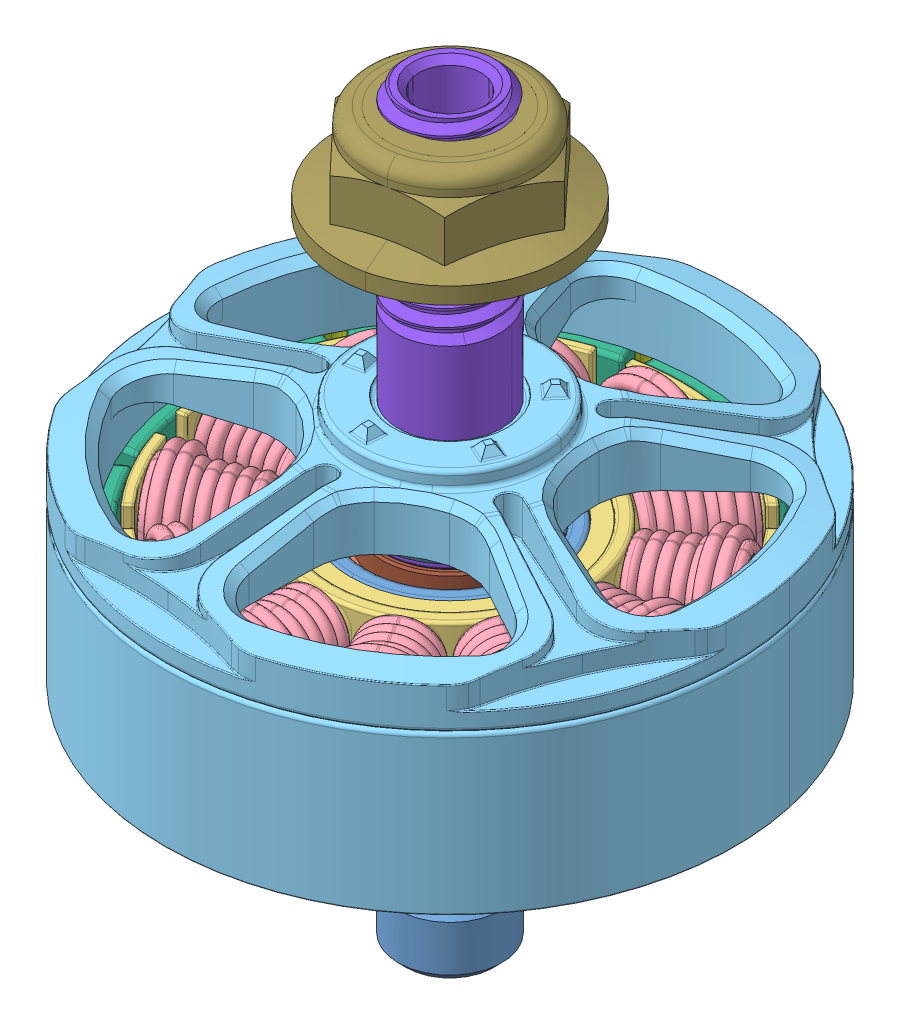
SolidWorks assembly EMAX RSII-2206 2300kv, configuration Default. Lengths in mm.
Overall size (32.76 30.2 32.81).
28 component instances, 13 part files, 0 mates.
Components (placement in the parent):
- EMAX RSII-2206 2300kv.STEP-1: EMAX RSII-2206 2300kv.STEP [Default] at origin size (61.91 30.2 32.81)
  - STATOR RSII-2206.STEP-1: STATOR RSII-2206.STEP [Default] at origin size (22.5 13.11 22.5)
    - STATOR BASE RSII-2206.STEP-1: STATOR BASE RSII-2206.STEP [Default] at origin size (16.31 12 16.31)
    - 3x8x4mm BEARING.STEP-1: 3x8x4mm BEARING.STEP [Default] at (0 5.3 0) x (1 0 0) z (0 0 -1) size (8 3 8)
    - 3x8x4mm BEARING.STEP-2: 3x8x4mm BEARING.STEP [Default] at (0 11 0) x (-0.982082 0 -0.188455) z (-0.188455 0 0.982082) size (8 3 8)
    - STATOR SLEEVE RSII-2206.STEP-1: STATOR SLEEVE RSII-2206.STEP [Default] at (0 5.5 0) size (22.5 6.65 22.5)
    - WINDING RSII-2206.STEP-1: WINDING RSII-2206.STEP [Default] at (8.5609 8.825 0) size (4.26 8.58 4.68)
    - WINDING RSII-2206.STEP-2: WINDING RSII-2206.STEP [Default] at (7.414 8.825 4.2805) x (0.866025 0 0.5) z (-0.5 0 0.866025) size (4.26 8.58 4.68)
    - WINDING RSII-2206.STEP-3: WINDING RSII-2206.STEP [Default] at (4.2805 8.825 7.414) x (0.5 0 0.866025) z (-0.866025 0 0.5) size (4.26 8.58 4.68)
    - WINDING RSII-2206.STEP-4: WINDING RSII-2206.STEP [Default] at (0 8.825 8.5609) x (0 0 1) z (-1 0 0) size (4.26 8.58 4.68)
    - WINDING RSII-2206.STEP-5: WINDING RSII-2206.STEP [Default] at (-4.2805 8.825 7.414) x (-0.5 0 0.866025) z (-0.866025 0 -0.5) size (4.26 8.58 4.68)
    - WINDING RSII-2206.STEP-6: WINDING RSII-2206.STEP [Default] at (-7.414 8.825 4.2805) x (-0.866025 0 0.5) z (-0.5 0 -0.866025) size (4.26 8.58 4.68)
    - WINDING RSII-2206.STEP-7: WINDING RSII-2206.STEP [Default] at (-8.5609 8.825 0) x (-1 0 0) z (0 0 -1) size (4.26 8.58 4.68)
    - WINDING RSII-2206.STEP-8: WINDING RSII-2206.STEP [Default] at (-7.414 8.825 -4.2805) x (-0.866025 0 -0.5) z (0.5 0 -0.866025) size (4.26 8.58 4.68)
    - WINDING RSII-2206.STEP-9: WINDING RSII-2206.STEP [Default] at (-4.2805 8.825 -7.414) x (-0.5 0 -0.866025) z (0.866025 0 -0.5) size (4.26 8.58 4.68)
    - WINDING RSII-2206.STEP-10: WINDING RSII-2206.STEP [Default] at (0 8.825 -8.5609) x (0 0 -1) z (1 0 0) size (4.26 8.58 4.68)
    - WINDING RSII-2206.STEP-11: WINDING RSII-2206.STEP [Default] at (4.2805 8.825 -7.414) x (0.5 0 -0.866025) z (0.866025 0 0.5) size (4.26 8.58 4.68)
    - WINDING RSII-2206.STEP-12: WINDING RSII-2206.STEP [Default] at (7.414 8.825 -4.2805) x (0.866025 0 -0.5) z (0.5 0 0.866025) size (4.26 8.58 4.68)
  - ROTOR RSII-2206.STEP-1: ROTOR RSII-2206.STEP [Default] x (-0.213902 0 -0.976855) z (0.976855 0 -0.213902) size (27.57 27.91 27.5)
    - ROTOR BELL RSII-2206.STEP-1: ROTOR BELL RSII-2206.STEP [Default] at origin size (27.57 12.4 27.5)
    - MAGNETS RSII-2206.STEP-1: MAGNETS RSII-2206.STEP [Default] at (0 5.8 0) size (25.73 6.01 25.8)
    - MAGNETS ADHESIVE RSII-2206.STEP-1: MAGNETS ADHESIVE RSII-2206.STEP [Default] at (0 5.9 0) size (26 5.9 26)
    - ROTOR SHAFT RSII-2206.STEP-1: ROTOR SHAFT RSII-2206.STEP [Default] at (0 2.3 0) size (6.5 27.91 6.5)
  - WASHER RSII-2206.STEP-1: WASHER RSII-2206.STEP [Default] at (0 1.7 0) x (0.649982 0 0.75995) z (-0.75995 0 0.649982) size (5 0.6 5)
  - SCREW_ROSCADO.STEP-1: SCREW_ROSCADO.STEP [Default] at (0 5.7 0) x (0 1 0) z (-0.487492 0 -0.873128) size (5.11 3.8 3.8)
  - MOTOR WIRES RSII-2206.STEP-1: MOTOR WIRES RSII-2206.STEP [Default] at (27 0.5 0) x (0 0 1) z (-1 0 0) size (11.02 5.99 39.03) (hidden)
  - SHAFT WASHER RSII-2206.STEP-1: SHAFT WASHER RSII-2206.STEP [Default] at (0 11 0) x (0.039546 0 0.999218) z (-0.999218 0 0.039546) size (6.7 1.1 6.7)
  - Low profile M5 lock nut.STEP-1: Low profile M5 lock nut.STEP [Default] at (0 28.2577 0) x (0.219878 0 0.975527) z (0 1 0) size (10.8 10.8 4.5)
